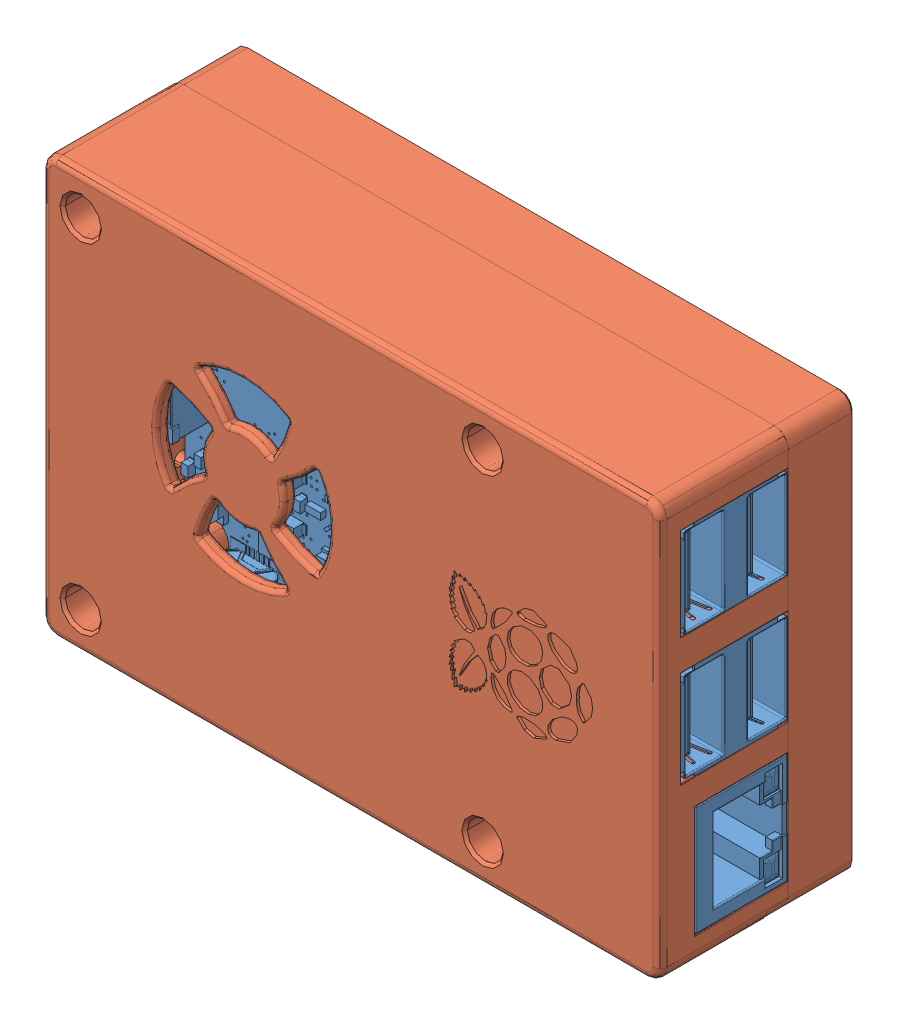
SolidWorks assembly Assembly_RaspberryPi_V1, configuration Défaut. Lengths in mm.
Overall size (89.18 60.77 28.17).
2 component instances, 2 part files, 3 mates.
Components (placement in the parent):
- raspberryPi3B-1: raspberryPi3B [Detailed] at (50.1305 49.7137 43.9055) size (87.05 58.5 19.5)
- RPI 3 B case.stp-1: RPI 3 B case.stp [Défaut] at (50.0883 49.899 43.6055) size (89.17 59.96 28.17)
Mates (geometry in assembly coordinates):
- Coincident7: coincident anti-aligned: plane of raspberryPi3B-1 through (50.1305 49.7137 45.2055) normal (0 0 -1); plane of RPI 3 B case.stp-1 through (7.5883 49.899 45.2055) normal (0 0 1)
- Coincident8: coincident anti-aligned: plane of raspberryPi3B-1 through (73.3305 39.9637 58.5055) normal (0 1 0); plane of RPI 3 B case.stp-1 through (92.7883 39.9637 51.9555) normal (0 -1 0)
- Coincident9: coincident anti-aligned: plane of raspberryPi3B-1 through (47.1305 31.7137 51.7055) normal (1 0 0); plane of RPI 3 B case.stp-1 through (47.1305 30.8824 44.5367) normal (-1 0 0)
